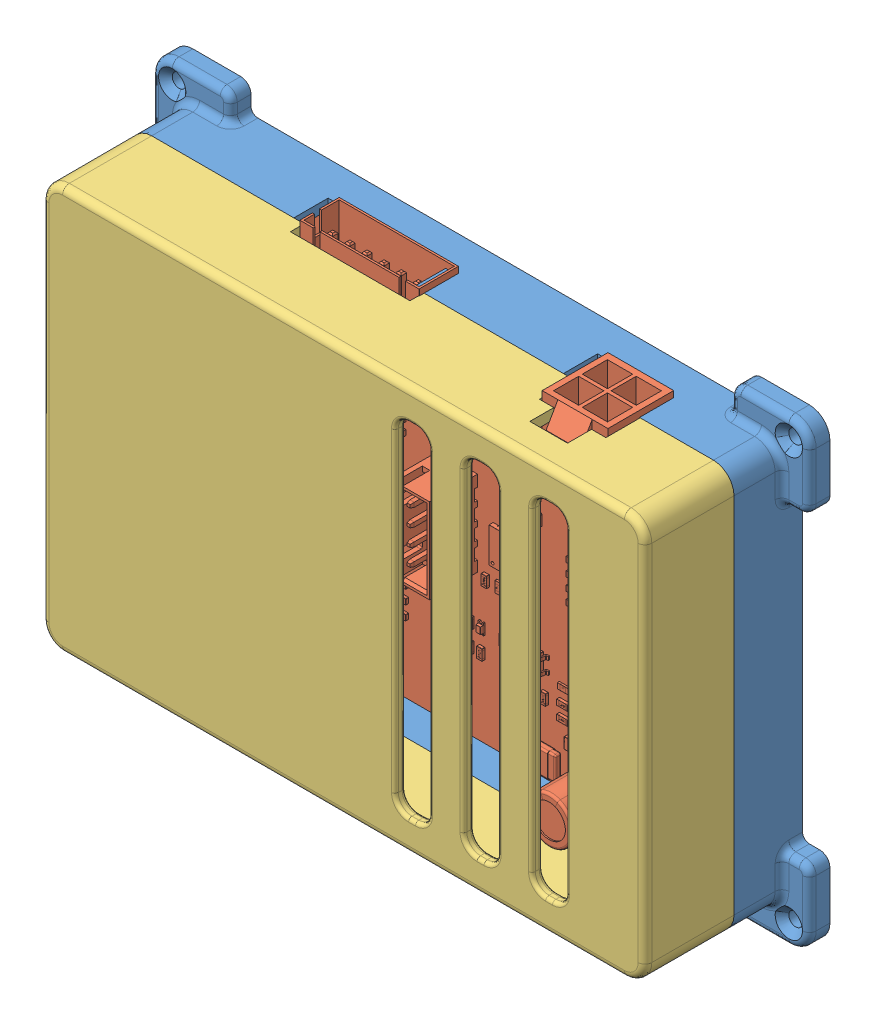
SolidWorks assembly case_RevA1, configuration По умолчанию. Lengths in mm.
Overall size (96 67 23).
3 component instances, 3 part files, 9 mates.
Components (placement in the parent):
- case_bottom-1: case_bottom [По умолчанию] at origin size (96 67 10)
- pcb-1: pcb [По умолчанию] at (-42.5 -28 5) size (87.4 58.4 16.61)
- case_top-1: case_top [По умолчанию] at origin size (88 59 21.56)
Mates (geometry in assembly coordinates):
- Coincident1: coincident: plane of case_bottom-1 through (-39.5 -28 3) normal (0 1 0); plane of pcb-1 through (39.5 -28 3.7086) normal (0 -1 0)
- Coincident2: coincident: plane of case_bottom-1 through (42.5 -25 3) normal (-1 0 0); plane of pcb-1 through (42.5 25 3.7086) normal (1 0 0)
- Coincident3: coincident: plane of case_bottom-1 through (-41 20.3 5) normal (0 0 1); plane of pcb-1 through (-38.4999 11.2999 5) normal (0 0 -1)
- Coincident4: coincident: plane of case_bottom-1 through (0 0 10) normal (0 0 1); plane of case_top-1 through (0 0 10) normal (0 0 -1)
- Coincident5: coincident: plane of case_bottom-1 through (0 0 10) normal (0 0 1); plane of case_top-1 through (0 0 10) normal (0 0 -1)
- Coincident6: coincident: plane of case_bottom-1 through (0 0 10) normal (0 0 1); plane of case_top-1 through (0 0 10) normal (0 0 -1)
- Coincident7: coincident: plane of case_bottom-1 through (0 0 10) normal (0 0 1); plane of case_top-1 through (0 0 10) normal (0 0 -1)
- Coincident8: coincident: plane of case_bottom-1 through (41 -29.5 23) normal (0 -1 0); plane of case_top-1 through (41 -29.5 23) normal (0 -1 0)
- Coincident9: coincident: plane of case_bottom-1 through (-44 -26.5 23) normal (-1 0 0); plane of case_top-1 through (-44 -26.5 23) normal (-1 0 0)
